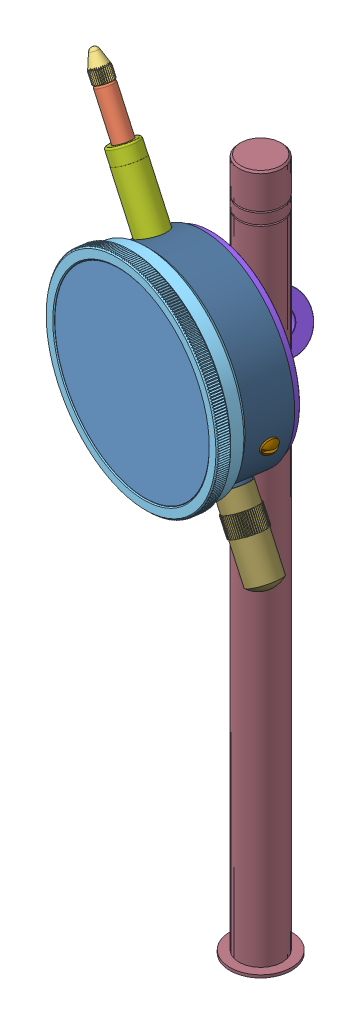
SolidWorks assembly dial on rod side, configuration Default. Lengths in mm.
Overall size (1000.28 216.66 622.85).
17 component instances, 13 part files, 0 mates.
Components (placement in the parent):
- Dial indicator - Mitutoyo NO.2046.step-1: Dial indicator - Mitutoyo NO.2046.step [Default] at (-2.8551 175.8539 9.3821) x (-0.854316 -0.500634 -0.139674) z (0.495819 -0.865606 0.069922) size (57.45 42.2 113.3)
  - Glass.step-1: Glass.step [Default] at (0 -18.65 0) x (0 0 1) z (-1 0 0) size (51.5 1.75 51.5)
  - Shaft.step-1: Shaft.step [Default] at (0 -5.75 29) size (6 6 90.9)
  - Tip.step-1: Tip.step [Default] at (0 -5.75 -52.3) size (5 5 12.5)
  - Back screw.step-1: Back screw.step [Default] at (16.2988 -3.2 -16.2988) x (0.707107 0 0.707107) z (0 1 0) size (3 3 5)
  - Dial.step-1: Dial.step [Default] at (0 -15.1 0) size (57.45 8.05 57.45)
  - Back screw.step-2: Back screw.step [Default] at (-16.2988 -3.2 -16.2988) x (0.707107 0 -0.707107) z (0 1 0) size (3 3 5)
  - Back screw.step-3: Back screw.step [Default] at (-16.2988 -3.2 16.2988) x (0.707107 0 0.707107) z (0 1 0) size (3 3 5)
  - Knurled screw.step-1: Knurled screw.step [Default] at (15.9356 -5.75 15.9356) x (0.707107 0 -0.707107) z (0.707107 0 0.707107) size (8.17 8.17 10.7)
  - Stem.step-1: Stem.step [Default] at (0 -5.85 -45.0423) size (7.9 7.9 24)
  - Back screw.step-4: Back screw.step [Default] at (16.2988 -3.2 16.2988) x (-0.707107 0 0.707107) z (0 1 0) size (3 3 5)
  - Back cover and lug.step-1: Back cover and lug.step [Default] x (1 0 0) z (0 0 -1) size (50.2 21.55 50.2)
  - M2.5x3.7.step-1: M2.5x3.7.step [Default] at (-19.6479 -5.75 19.6479) x (-0.707107 0 -0.707107) z (-0.707107 0 0.707107) size (4.4 4.4 5.4)
  - Case.step-1: Case.step [Default] at origin size (52 15.1 55.04)
  - Long pointer.step-1: Long pointer.step [Default] at (0 -18.6 0) x (0.431825 0 0.901957) z (-0.901957 0 0.431825) size (3.8 6.56 25.9)
  - Cover knob.step-1: Cover knob.step [Default] at (0 -5.75 26.5) size (8.99 8.99 22)
- rod-2: rod [2310A15] at origin size (1000.28 191.26 622.85)
